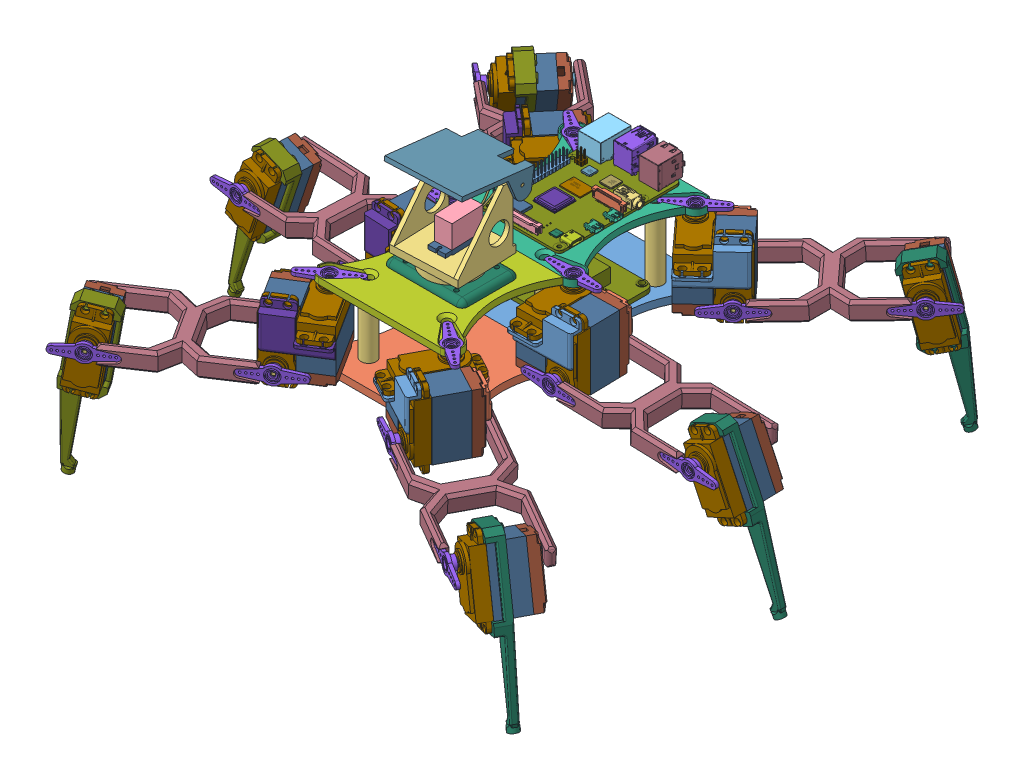
SolidWorks assembly 初号机, configuration 默认. Lengths in mm. (continued)
Components (placement in the parent): (continued)
- 舵机驱动板示意图-2: 舵机驱动板示意图 [默认] at (1.8543 8 4.9136) size (65 13 55)
Mates (geometry in assembly coordinates):
- 同心2: concentric anti-aligned: circle of bottom.step-1/Основание нижнее-0.step-1; circle of Втулка опорная-1
- 重合2: coincident anti-aligned: plane of bottom^666-1/Основание нижнее-0^bottom_666-1 through (0 5 85) normal (0 1 0); plane of Втулка опорная-1 through (-26.5949 5 115.9923) normal (0 -1 0)
- 同心3: concentric aligned: circle of bottom.step-1/Основание нижнее.step-1; circle of Втулка опорная-2
- 重合3: coincident anti-aligned: plane of bottom^666-1/Основание нижнее-0^bottom_666-1 through (0 5 85) normal (0 1 0); plane of Втулка опорная-2 through (-22.868 5 42.5) normal (0 -1 0)
- 重合4: coincident anti-aligned: plane of bottom^666-1/Основание нижнее^bottom_666-1 through (0 5 0) normal (0 1 0); plane of Втулка опорная-3 through (-26.5949 5 -30.9923) normal (0 -1 0)
- 同心5: concentric anti-aligned: cylinder of bottom.step-1/Основание нижнее.step-1; cylinder of Втулка опорная-3 through (-26.5949 50 -30.9923) axis (0 -1 0) radius 5.2
- 同心6: concentric aligned: circle of bottom.step-1/Основание нижнее.step-1; circle of Втулка опорная-4
- 重合5: coincident anti-aligned: plane of bottom^666-1/Основание нижнее^bottom_666-1 through (0 5 0) normal (0 1 0); plane of Втулка опорная-4 through (27.1009 5 -30.1473) normal (0 -1 0)
- 同心8: concentric anti-aligned: cylinder of bottom^666-1/Основание нижнее-0^bottom_666-1 through (27.1009 5 115.1473) axis (0 -1 0) radius 3; circle of Втулка опорная-6
- 重合6: coincident anti-aligned: plane of bottom^666-1/Основание нижнее-0^bottom_666-1 through (0 5 85) normal (0 1 0); plane of Втулка опорная-6 through (27.1009 5 115.1473) normal (0 -1 0)
- 重合7: coincident anti-aligned: plane of bottom^666-1/Основание нижнее^bottom_666-1 through (0 5 0) normal (0 1 0); plane of Втулка опорная-5 through (22.868 5 42.5) normal (0 -1 0)
- 同心9: concentric aligned: circle of Втулка опорная-5; circle of bottom.step-1/Основание нижнее.step-1
- 在位2: in place: plane of ? through (0 5 0) normal (0 1 0); plane of 零件4^初号机-1 through (0 5 0) normal (0 1 0); moOrthogonalPlaneRef_w of ? through (0 5 0) normal (0 1 0); plane of 零件4^初号机-1 through (0 5 0) normal (0 0 -1); plane of ? through (0 5 0) normal (0 1 0); plane of 零件4^初号机-1 through (0 5 0) normal (1 0 0); plane of ? through (0 5 0) normal (0 1 0); unknown of 零件4^初号机-1
- 重合21: coincident aligned: plane of ?; plane of ?
- 重合22: coincident aligned: moOrthogonalPlaneRef_w of bottom^666-1/Основание нижнее^bottom_666-1 through (0 5 0) normal (0 0 -1); plane of 零件4^666-1 through (0 5 0) normal (0 0 -1)
- 重合23: coincident anti-aligned: moOrthogonalPlaneRef_w of bottom^666-1/Основание нижнее^bottom_666-1 through (0 5 0) normal (-1 0 0); plane of 零件4^666-1 through (0 5 0) normal (1 0 0)
- 在位3: in place: plane of ? through (0 0 0) normal (0 -1 0); plane of 零件5^初号机-1 through (0 0 0) normal (0 -1 0); plane of ? through (0 0 0) normal (0 -1 0); plane of 零件5^初号机-1 through (0 0 0) normal (0 0 -1); plane of ? through (0 0 0) normal (0 -1 0); plane of 零件5^初号机-1 through (0 0 0) normal (-1 0 0); plane of ? through (0 0 0) normal (0 -1 0); unknown of 零件5^初号机-1
- 重合28: coincident aligned: plane of ?; plane of ?
- 重合29: coincident aligned: moOrthogonalPlaneRef_w of bottom^666-1/Основание нижнее^bottom_666-1 through (0 0 0) normal (0 0 -1); plane of 零件5^666-1 through (0 0 0) normal (0 0 -1)
- 重合30: coincident anti-aligned: moOrthogonalPlaneRef_w of bottom^666-1/Основание нижнее^bottom_666-1 through (0 0 0) normal (1 0 0); plane of 零件5^666-1 through (0 0 0) normal (-1 0 0)
- 同心10: concentric anti-aligned: cylinder of Втулка площадки-1 through (-42.5 5.3 -42.5) axis (0 -1 0) radius 2.5; circle of Подшипник-1
- 重合31: coincident anti-aligned: plane of Втулка площадки-1 through (-42.5 5.3 -42.5) normal (0 -1 0); circle of Подшипник-1
- 同心11: concentric aligned: circle of bottom^666-1/Основание нижнее^bottom_666-1; circle of Втулка площадки-1
- 重合33: coincident anti-aligned: plane of bottom^666-1/Основание нижнее^bottom_666-1 through (-42.5 3 -42.5) normal (0 1 0); plane of Подшипник-1 through (-42.5 3 -42.5) normal (0 -1 0)
- 同心12: concentric aligned: circle of Втулка площадки-2; circle of Подшипник-2
- 重合35: coincident anti-aligned: plane of Втулка площадки-2 through (42.5 5.5 -42.5) normal (0 -1 0); plane of Подшипник-2 through (42.5 5.5 -42.5) normal (0 1 0)
- 同心13: concentric aligned: circle of bottom^666-1/Основание нижнее^bottom_666-1; circle of Втулка площадки-2
- 重合36: coincident anti-aligned: plane of bottom^666-1/Основание нижнее^bottom_666-1 through (42.5 3 -42.5) normal (0 1 0); plane of Подшипник-2 through (42.5 3 -42.5) normal (0 -1 0)
- 同心14: concentric aligned: circle of Втулка площадки-3; circle of Подшипник-3
- 重合37: coincident anti-aligned: plane of Втулка площадки-3 through (42.5 7.5 42.5) normal (0 -1 0); plane of Подшипник-3 through (42.5 7.5 42.5) normal (0 1 0)
- 同心15: concentric aligned: circle of bottom^666-1/Основание нижнее^bottom_666-1; circle of Подшипник-3
- 重合38: coincident anti-aligned: plane of bottom^666-1/Основание нижнее-0^bottom_666-1 through (0 5 85) normal (0 1 0); plane of Подшипник-3 through (42.5 5 42.5) normal (0 -1 0)
- 同心17: concentric aligned: circle of bottom^666-1/Основание нижнее-0^bottom_666-1; circle of 底板转柱-4
- 同心18: concentric aligned: circle of bottom^666-1/Основание нижнее-0^bottom_666-1; circle of Подшипник-4
- 重合40: coincident anti-aligned: plane of 底板转柱-4 through (42.5 5.5 127.5) normal (0 -1 0); plane of Подшипник-4 through (42.5 5.5 127.5) normal (0 1 0)
- 重合41: coincident anti-aligned: plane of bottom^666-1/Основание нижнее-0^bottom_666-1 through (42.5 3 127.5) normal (0 1 0); plane of Подшипник-4 through (42.5 3 127.5) normal (0 -1 0)
- 同心19: concentric aligned: circle of 底板转柱-5; circle of Подшипник-6
- 重合43: coincident anti-aligned: plane of 底板转柱-5 through (-42.5 5.3 127.5) normal (0 -1 0); plane of Подшипник-6 through (-42.5 5.3 127.5) normal (0 1 0)
- 同心20: concentric aligned: circle of bottom^666-1/Основание нижнее-0^bottom_666-1; circle of 底板转柱-5
- 重合44: coincident anti-aligned: plane of bottom^666-1/Основание нижнее-0^bottom_666-1 through (-42.5 3 127.5) normal (0 1 0); plane of Подшипник-6 through (-42.5 3 127.5) normal (0 -1 0)
- 同心21: concentric aligned: circle of Подшипник-5; circle of 底板转柱-6
- 重合45: coincident anti-aligned: plane of Подшипник-5 through (-42.5 5.5 42.5) normal (0 1 0); plane of 底板转柱-6 through (-42.5 5.5 42.5) normal (0 -1 0)
- 同心22: concentric aligned: circle of Подшипник-5; circle of bottom^666-1/Основание нижнее^bottom_666-1
- 重合46: coincident anti-aligned: plane of bottom^666-1/Основание нижнее^bottom_666-1 through (-42.5 3 42.5) normal (0 1 0); plane of Подшипник-5 through (-42.5 3 42.5) normal (0 -1 0)
- 同心36: concentric anti-aligned: circle of Рычаг-7; circle of Servo MG955-1/Втулка-1
- 重合72: coincident anti-aligned: plane of Рычаг-7 through (-42.5 51.5 127.5) normal (0 -1 0); plane of Servo MG955-1/MG995齿轮-1 through (-42.5 51.5 127.5) normal (0 1 0)
- 重合83: coincident anti-aligned: plane of Servo MG955-1/MG995中板-1 through (-56.5553 34.5 124.2521) normal (-0.84292 0 0.538039); plane of 腿1-2/Servo MG955-2/MG995中板-1 through (-40.6024 4.85 149.2447) normal (0.84292 0 -0.538039)
- 重合84: coincident aligned: plane of Servo MG955-1/MG995中板-1 through (-34.6302 34.5 158.6011) normal (0.538039 0 0.84292); plane of 腿1-2/Servo MG955-2/MG995前板-1 through (-43.1437 35.4 164.0353) normal (0.538039 0 0.84292)
- 重合85: coincident aligned: plane of Servo MG955-1/MG995前板-1 through (-31.6047 45.6 144.5691) normal (0 1 0); plane of 腿1-2/Servo MG955-2/MG995中板-1 through (-40.6024 45.6 149.2447) normal (0 1 0)
- 重合86: coincident anti-aligned: plane of 底板支柱-4 through (27.1009 50 -30.1473) normal (0 1 0); plane of top(3)-1/top(3)^top(3)-2/^top(3)_top(3)-1/Основание нижнее^_top(3)_top(3)-1 through (0 50 0) normal (0 -1 0)
- 同心37: concentric anti-aligned: circle of 底板支柱-4; circle of top(3)-1/top(3)^top(3)-2/^top(3)_top(3)-1/Основание нижнее^_top(3)_top(3)-1
- 同心38: concentric anti-aligned: circle of 底板支柱-1; circle of top(3)-1/top(3)^top(3)-2/_private_var_mobile_Containers_Data_Application_327FD876-EF9E-4CCE-9D75-9D16AF0753A7_tmp_B33AE067-E3AF-4F21-8502-7502B160869B.tmp(2)^top(3)_top(3)-1
- 同心39: concentric aligned: circle of top(3)-1/top(3)^top(3)-2/_private_var_mobile_Containers_Data_Application_327FD876-EF9E-4CCE-9D75-9D16AF0753A7_tmp_B33AE067-E3AF-4F21-8502-7502B160869B.tmp(2)^top(3)_top(3)-1; circle of 舵机配件-7
- 重合87: coincident anti-aligned: plane of top(3)-1/top(3)^top(3)-2/_private_var_mobile_Containers_Data_Application_327FD876-EF9E-4CCE-9D75-9D16AF0753A7_tmp_B33AE067-E3AF-4F21-8502-7502B160869B.tmp(2)^top(3)_top(3)-1 through (0 51.5 0) normal (0 1 0); plane of 舵机配件-7 through (-42.5 51.5 127.5) normal (0 -1 0)
- 平行1: parallel aligned: line of top(3)-1/top(3)^top(3)-2/_private_var_mobile_Containers_Data_Application_327FD876-EF9E-4CCE-9D75-9D16AF0753A7_tmp_B33AE067-E3AF-4F21-8502-7502B160869B.tmp(2)^top(3)_top(3)-1 through (-42.5 51.5 127.5) axis (0.81018 0 -0.586182); line of 舵机配件-7 through (-55.8921 53.8 137.1895) axis (0.81018 0 -0.586182)
- 同心40: concentric aligned: circle of top(3)-1/top(3)^top(3)-2/_private_var_mobile_Containers_Data_Application_327FD876-EF9E-4CCE-9D75-9D16AF0753A7_tmp_B33AE067-E3AF-4F21-8502-7502B160869B.tmp(2)^top(3)_top(3)-1; circle of 舵机配件-6
- 重合89: coincident anti-aligned: plane of top(3)-1/top(3)^top(3)-2/_private_var_mobile_Containers_Data_Application_327FD876-EF9E-4CCE-9D75-9D16AF0753A7_tmp_B33AE067-E3AF-4F21-8502-7502B160869B.tmp(2)^top(3)_top(3)-1 through (0 51.5 0) normal (0 1 0); plane of 舵机配件-6 through (42.5 51.5 127.5) normal (0 -1 0)
- 平行2: parallel aligned: line of top(3)-1/top(3)^top(3)-2/_private_var_mobile_Containers_Data_Application_327FD876-EF9E-4CCE-9D75-9D16AF0753A7_tmp_B33AE067-E3AF-4F21-8502-7502B160869B.tmp(2)^top(3)_top(3)-1 through (34.4656 51.5 121.055) axis (0.780043 0 0.625726); line of 舵机配件-6 through (29.6061 53.8 117.1569) axis (0.780043 0 0.625726)
- 同心41: concentric aligned: circle of top(3)-1/top(3)^top(3)-2/^top(3)_top(3)-1/Основание нижнее^_top(3)_top(3)-1; circle of 舵机配件-8
- 重合91: coincident anti-aligned: plane of top(3)-1/top(3)^top(3)-2/^top(3)_top(3)-1/Основание нижнее^_top(3)_top(3)-1 through (0 51.5 0) normal (0 1 0); plane of 舵机配件-8 through (42.5 51.5 42.5) normal (0 -1 0)
- 平行3: parallel aligned: line of top(3)-1/top(3)^top(3)-2/^top(3)_top(3)-1/Основание нижнее^_top(3)_top(3)-1 through (42.5 51.5 42.5) axis (-1 0 0); line of 舵机配件-8 through (59.0298 53.8 42.5) axis (-1 0 0)
- 同心42: concentric anti-aligned: circle of top(3)-1/top(3)^top(3)-2/^top(3)_top(3)-1/Основание нижнее^_top(3)_top(3)-1; circle of 舵机配件-5
- 重合95: coincident anti-aligned: plane of top(3)-1/top(3)^top(3)-2/^top(3)_top(3)-1/Основание нижнее^_top(3)_top(3)-1 through (0 51.5 0) normal (0 1 0); plane of 舵机配件-5 through (-42.5 51.5 42.5) normal (0 -1 0)
- 平行4: parallel aligned: line of top(3)-1/top(3)^top(3)-2/^top(3)_top(3)-1/Основание нижнее^_top(3)_top(3)-1 through (-42.5 51.5 42.5) axis (1 0 0); line of 舵机配件-5 through (-59.0298 53.8 42.5) axis (1 0 0)
- 同心44: concentric aligned: circle of top(3)-1/top(3)^top(3)-2/^top(3)_top(3)-1/Основание нижнее^_top(3)_top(3)-1; circle of 舵机配件-4
- 重合97: coincident anti-aligned: plane of top(3)-1/top(3)^top(3)-2/^top(3)_top(3)-1/Основание нижнее^_top(3)_top(3)-1 through (0 51.5 0) normal (0 1 0); plane of 舵机配件-4 through (-42.5 51.5 -42.5) normal (0 -1 0)
- 平行5: parallel aligned: line of top(3)-1/top(3)^top(3)-2/^top(3)_top(3)-1/Основание нижнее^_top(3)_top(3)-1 through (-42.5 51.5 -42.5) axis (0.81018 0 0.586182); line of 舵机配件-4 through (-55.8921 53.8 -52.1895) axis (0.81018 0 0.586182)
- 同心45: concentric aligned: circle of top(3)-1/top(3)^top(3)-2/^top(3)_top(3)-1/Основание нижнее^_top(3)_top(3)-1; circle of 舵机配件-3
- 重合99: coincident anti-aligned: plane of top(3)-1/top(3)^top(3)-2/^top(3)_top(3)-1/Основание нижнее^_top(3)_top(3)-1 through (0 51.5 0) normal (0 1 0); plane of 舵机配件-3 through (42.5 51.5 -42.5) normal (0 -1 0)
- 平行6: parallel anti-aligned: line of top(3)-1/top(3)^top(3)-2/^top(3)_top(3)-1/Основание нижнее^_top(3)_top(3)-1 through (42.5 51.5 -42.5) axis (-0.783045 0 0.621965); line of 舵机配件-3 through (29.5564 53.8 -32.2191) axis (0.783045 0 -0.621965)
- 重合100: coincident anti-aligned: plane of 腿1-2/Servo MG955-2/MG995前板-1 through (-43.1437 35.4 164.0353) normal (0.538039 0 0.84292); plane of 固定件1-1 through (-26.1167 13.85 153.1669) normal (-0.538039 0 -0.84292)
- 同心46: concentric aligned: circle of 腿1-2/Servo MG955-2/MG995前板-1; circle of 固定件1-1
- 重合102: coincident anti-aligned: line of Servo MG955-1/MG995中板-1 through (-34.6302 34.5 158.6011) axis (0.84292 0 -0.538039); line of 固定件1-1 through (-17.6032 34.5 147.7327) axis (-0.84292 0 0.538039)
- 重合103: coincident anti-aligned: plane of 腿1-2/Servo MG955-2/MG995后板-1 through (-64.2348 25.235 130.9928) normal (-0.538039 0 -0.84292); plane of 固定件2-1 through (-47.2078 13.85 120.1244) normal (0.538039 0 0.84292)
- 同心47: concentric aligned: circle of 腿1-2/Servo MG955-2/MG995后板-1; circle of 固定件2-1
- 同心48: concentric anti-aligned: circle of 腿1-2/Servo MG955-2/MG995后板-1; circle of 固定件2-1
- 重合106: coincident anti-aligned: plane of 舵机配件-5 through (-42.5 51.5 42.5) normal (0 -1 0); plane of Servo MG955-2/MG995齿轮-1 through (-42.5 51.5 42.5) normal (0 1 0)
- 同心49: concentric anti-aligned: circle of 舵机配件-5; circle of Servo MG955-2/MG995齿轮-1
- 重合107: coincident anti-aligned: plane of 腿1-3/Servo MG955-2/MG995中板-1 through (-53.5221 4.85 61.34) normal (0.998835 0 0.048264); plane of Servo MG955-2/MG995中板-1 through (-52.0911 34.5 31.7245) normal (-0.998835 0 -0.048264)
- 重合108: coincident aligned: plane of 腿1-3/Servo MG955-2/MG995前板-1 through (-64.1461 35.4 71.9396) normal (-0.048264 0 0.998835); plane of Servo MG955-2/MG995中板-1 through (-54.0579 34.5 72.4271) normal (-0.048264 0 0.998835)
- 重合109: coincident aligned: plane of 腿1-3/Servo MG955-2/MG995中板-1 through (-53.5221 45.6 61.34) normal (0 1 0); plane of Servo MG955-2/MG995前板-1 through (-43.4773 45.6 62.7264) normal (0 1 0)
- 重合110: coincident anti-aligned: plane of 腿1-3/Servo MG955-2/MG995前板-1 through (-64.1461 35.4 71.9396) normal (-0.048264 0 0.998835); plane of 固定件1-2 through (-43.9696 13.85 72.9145) normal (0.048264 0 -0.998835)
- 同心50: concentric aligned: circle of 腿1-3/Servo MG955-2/MG995前板-1; circle of 固定件1-2
- 重合113: coincident anti-aligned: line of Servo MG955-2/MG995中板-1 through (-54.0579 34.5 72.4271) axis (0.998835 0 0.048264); line of 固定件1-2 through (-33.8814 34.5 73.402) axis (-0.998835 0 -0.048264)
- 同心51: concentric aligned: circle of 腿1-3/Servo MG955-2/MG995后板-1; circle of 固定件2-2
- 同心52: concentric anti-aligned: circle of 腿1-2/Servo MG955-2/MG995后板-1; circle of 固定件2-1
- 重合119: coincident anti-aligned: plane of 腿1-3/Servo MG955-2/MG995后板-1 through (-72.4075 45.6 33.6462) normal (0.048264 0 -0.998835); plane of 固定件2-2 through (-42.1428 13.85 35.1086) normal (-0.048264 0 0.998835)
- 同心54: concentric anti-aligned: circle of 腿1-3/Servo MG955-2/MG995后板-1; circle of 固定件2-2
- 重合126: coincident anti-aligned: plane of 腿1-4/Servo MG955-2/MG995前板-1 through (-77.5718 35.4 -32.2426) normal (-0.644628 0 0.764496); plane of 固定件1-3 through (-62.1289 13.85 -19.2211) normal (0.644628 0 -0.764496)
- 同心57: concentric aligned: circle of 腿1-4/Servo MG955-2/MG995前板-1; circle of 固定件1-3
- 同心58: concentric aligned: circle of 腿1-4/Servo MG955-2/MG995前板-1; circle of 固定件1-3
- 重合130: coincident anti-aligned: plane of 腿1-4/Servo MG955-2/MG995后板-1 through (-52.3023 25.235 -62.2108) normal (0.644628 0 -0.764496); plane of 固定件2-3 through (-36.8595 13.85 -49.1893) normal (-0.644628 0 0.764496)
- 同心59: concentric anti-aligned: circle of 腿1-4/Servo MG955-2/MG995后板-1; circle of 固定件2-3
- 同心60: concentric aligned: circle of 腿1-4/Servo MG955-2/MG995后板-1; circle of 固定件2-3
- 同心61: concentric anti-aligned: circle of 舵机配件-6; circle of Servo MG955-4/MG995齿轮-1
- 重合135: coincident anti-aligned: plane of 舵机配件-6 through (42.5 51.5 127.5) normal (0 -1 0); plane of Servo MG955-4/MG995齿轮-1 through (42.5 51.5 127.5) normal (0 1 0)
- 重合136: coincident anti-aligned: plane of Servo MG955-4/MG995中板-1 through (56.2471 34.5 123.1278) normal (0.883614 0 0.468216); plane of 腿2-2/Servo MG955-2/MG995中板-1 through (42.3645 4.85 149.3269) normal (-0.883614 0 -0.468216)
- 重合137: coincident aligned: plane of Servo MG955-4/MG995前板-1 through (33.0186 45.6 145.3932) normal (0 1 0); plane of 腿2-2/Servo MG955-2/MG995中板-1 through (60.2135 45.6 158.7849) normal (0 1 0)
- 重合138: coincident aligned: plane of Servo MG955-4/MG995中板-1 through (19.3183 34.5 149.6771) normal (-0.468216 0 0.883614); plane of 腿2-2/Servo MG955-2/MG995前板-1 through (46.0918 35.4 163.864) normal (-0.468216 0 0.883614)
- 重合139: coincident anti-aligned: plane of 腿2-2/Servo MG955-2/MG995前板-1 through (46.0918 35.4 163.864) normal (-0.468216 0 0.883614); plane of 镜向固定件1-1 through (28.2428 13.85 154.406) normal (0.468216 0 -0.883614)
- 同心62: concentric anti-aligned: circle of 腿2-2/Servo MG955-2/MG995前板-1; circle of 镜向固定件1-1
- 同心63: concentric anti-aligned: circle of 腿2-2/Servo MG955-2/MG995前板-1; circle of 镜向固定件1-1
- 重合143: coincident anti-aligned: plane of 腿2-2/Servo MG955-2/MG995后板-1 through (64.4459 25.235 129.2263) normal (0.468216 0 -0.883614); plane of 镜向固定件2-1 through (46.5969 13.85 119.7684) normal (-0.468216 0 0.883614)
- 同心64: concentric anti-aligned: circle of 腿2-2/Servo MG955-2/MG995后板-1; circle of 镜向固定件2-1
- 同心65: concentric aligned: circle of 腿2-2/Servo MG955-2/MG995后板-1; circle of 镜向固定件2-1
- 同心66: concentric anti-aligned: circle of 舵机配件-8; circle of Servo MG955-5/MG995齿轮-1
- 重合146: coincident anti-aligned: plane of 舵机配件-8 through (42.5 51.5 42.5) normal (0 -1 0); circle of Servo MG955-5/MG995齿轮-1
- 重合147: coincident anti-aligned: plane of 腿2-1/Servo MG955-2/MG995中板-1 through (53.0061 4.85 61.6325) normal (-0.999777 0 0.021104); plane of Servo MG955-5/MG995中板-1 through (52.3804 34.5 31.9891) normal (0.999777 0 -0.021104)
- 重合148: coincident aligned: plane of 腿2-1/Servo MG955-2/MG995前板-1 through (63.3381 35.4 72.5169) normal (0.021104 0 0.999777); plane of Servo MG955-5/MG995中板-1 through (33.0449 34.5 73.1564) normal (0.021104 0 0.999777)
- 重合149: coincident aligned: plane of 腿2-1/Servo MG955-2/MG995中板-1 through (73.2016 45.6 61.2062) normal (0 1 0); plane of Servo MG955-5/MG995前板-1 through (42.9274 45.6 62.7455) normal (0 1 0)
- 重合151: coincident anti-aligned: plane of 腿2-1/Servo MG955-2/MG995前板-1 through (63.3381 35.4 72.5169) normal (0.021104 0 0.999777); plane of 镜向固定件1-2 through (43.1426 13.85 72.9432) normal (-0.021104 0 -0.999777)
- 同心67: concentric anti-aligned: circle of 腿2-1/Servo MG955-2/MG995前板-1; circle of 镜向固定件1-2
- 同心68: concentric anti-aligned: circle of 腿2-1/Servo MG955-2/MG995前板-1; circle of 镜向固定件1-2
- 重合154: coincident anti-aligned: plane of 腿2-1/Servo MG955-2/MG995后板-1 through (62.5108 25.235 33.3256) normal (-0.021104 0 -0.999777); plane of 镜向固定件2-2 through (42.3153 13.85 33.7519) normal (0.021104 0 0.999777)
- 同心69: concentric aligned: circle of 腿2-1/Servo MG955-2/MG995后板-1; circle of 镜向固定件2-2
- 同心70: concentric anti-aligned: circle of 腿2-1/Servo MG955-2/MG995后板-1; circle of 镜向固定件2-2
- 重合157: coincident anti-aligned: plane of 舵机配件-3 through (42.5 51.5 -42.5) normal (0 -1 0); plane of Servo MG955-6/MG995齿轮-1 through (42.5 51.5 -42.5) normal (0 1 0)
- 同心71: concentric anti-aligned: circle of 舵机配件-3; circle of Servo MG955-6/MG995齿轮-1
- 重合158: coincident anti-aligned: plane of Servo MG955-6/MG995中板-1 through (43.0145 34.5 -56.9165) normal (0.73852 0 -0.674231); plane of 腿2-3/Servo MG955-2/MG995中板-1 through (63.0054 4.85 -35.0194) normal (-0.73852 0 0.674231)
- 重合159: coincident aligned: plane of Servo MG955-6/MG995中板-1 through (55.5713 34.5 -13.2023) normal (0.674231 0 0.73852); plane of 腿2-3/Servo MG955-2/MG995前板-1 through (77.9484 35.4 -33.6315) normal (0.674231 0 0.73852)
- 重合160: coincident aligned: plane of Servo MG955-6/MG995前板-1 through (56.1532 45.6 -27.545) normal (0 1 0); plane of 腿2-3/Servo MG955-2/MG995中板-1 through (77.9235 45.6 -48.6388) normal (0 1 0)
- 重合161: coincident anti-aligned: plane of 腿2-3/Servo MG955-2/MG995前板-1 through (77.9484 35.4 -33.6315) normal (0.674231 0 0.73852); plane of 镜向固定件1-3 through (63.0303 13.85 -20.0121) normal (-0.674231 0 -0.73852)
- 同心72: concentric anti-aligned: circle of 腿2-3/Servo MG955-2/MG995前板-1; circle of 镜向固定件1-3
- 同心73: concentric anti-aligned: circle of 腿2-3/Servo MG955-2/MG995前板-1; circle of 镜向固定件1-3
- 重合165: coincident aligned: plane of Servo MG955-4/MG995前板-1 through (33.0186 45.6 145.3932) normal (0 1 0); plane of 腿2-2/Servo MG955-2/MG995中板-1 through (60.2135 45.6 158.7849) normal (0 1 0)
- 平行9: parallel anti-aligned: plane of Servo MG955-4/MG995中板-1 through (56.2471 34.5 123.1278) normal (0.883614 0 0.468216); plane of 腿2-2/Servo MG955-2/MG995中板-1 through (42.3645 4.85 149.3269) normal (-0.883614 0 -0.468216)
- 重合169: coincident anti-aligned: plane of Servo MG955-4/MG995中板-1 through (56.2471 34.5 123.1278) normal (0.883614 0 0.468216); plane of 腿2-2/Servo MG955-2/MG995中板-1 through (42.3645 4.85 149.3269) normal (-0.883614 0 -0.468216)
- 重合170: coincident anti-aligned: plane of 腿2-3/Servo MG955-2/MG995后板-1 through (51.5186 25.235 -62.5815) normal (-0.674231 0 -0.73852); plane of 镜向固定件2-3 through (36.6005 13.85 -48.9621) normal (0.674231 0 0.73852)
- 同心74: concentric aligned: circle of 腿2-3/Servo MG955-2/MG995后板-1; circle of 镜向固定件2-3
- 同心75: concentric anti-aligned: circle of 腿2-3/Servo MG955-2/MG995后板-1; circle of 镜向固定件2-3
- 重合173: coincident anti-aligned: plane of 舵机配件-4 through (-42.5 51.5 -42.5) normal (0 -1 0); plane of Servo MG955-7/MG995齿轮-1 through (-42.5 51.5 -42.5) normal (0 1 0)
- 同心76: concentric aligned: circle of 舵机配件-4; circle of Servo MG955-7/MG995齿轮-1
- 重合174: coincident anti-aligned: plane of 腿1-4/Servo MG955-2/MG995中板-1 through (-62.695 4.85 -34.2177) normal (0.764496 0 0.644628); plane of Servo MG955-7/MG995中板-1 through (-43.5817 34.5 -56.8851) normal (-0.764496 0 -0.644628)
- 重合175: coincident aligned: plane of 腿1-4/Servo MG955-2/MG995中板-1 through (-62.695 45.6 -34.2177) normal (0 1 0); plane of Servo MG955-7/MG995前板-1 through (-55.5537 45.6 -27.0189) normal (0 1 0)
- 重合177: coincident anti-aligned: plane of 固定件1-3 through (-62.1289 13.85 -19.2211) normal (0.644628 0 -0.764496); plane of Servo MG955-7/MG995中板-1 through (-69.8503 34.5 -25.7318) normal (-0.644628 0 0.764496)
- 重合178: coincident anti-aligned: plane of top(3)-1/top(3)^top(3)-2/_private_var_mobile_Containers_Data_Application_327FD876-EF9E-4CCE-9D75-9D16AF0753A7_tmp_B33AE067-E3AF-4F21-8502-7502B160869B.tmp(2)^top(3)_top(3)-1 through (0 55 85) normal (0 1 0); plane of 云台2号机 -1/云台1-1 through (0 55 85) normal (0 -1 0)
- 重合182: coincident anti-aligned: line of top(3)-1/top(3)^top(3)-2/_private_var_mobile_Containers_Data_Application_327FD876-EF9E-4CCE-9D75-9D16AF0753A7_tmp_B33AE067-E3AF-4F21-8502-7502B160869B.tmp(2)^top(3)_top(3)-1 through (-42.8869 55 85) axis (1 0 0); line of 云台2号机 -1/云台1-1 through (17.5 55 85) axis (-1 0 0)
- 重合183: coincident aligned: line of top(3)-1/top(3)^top(3)-2/_private_var_mobile_Containers_Data_Application_327FD876-EF9E-4CCE-9D75-9D16AF0753A7_tmp_B33AE067-E3AF-4F21-8502-7502B160869B.tmp(2)^top(3)_top(3)-1 through (0 55 49.99) axis (0 0 1); line of 云台2号机 -1/云台1-1 through (0 55 71) axis (0 0 1)
- 重合187: coincident anti-aligned: plane of top(3)-1/top(3)^top(3)-2/^top(3)_top(3)-1/Основание нижнее^_top(3)_top(3)-1 through (0 55 0) normal (0 1 0); plane of rpi4b-1/rpi4b(2)^rpi4b-1/PCB, RPi4ModelB^rpi4b(2)_rpi4b-1 through (0 55 -4.664) normal (0 -1 0)
- 重合188: coincident aligned: line of top(3)-1/top(3)^top(3)-2/^top(3)_top(3)-1/Основание нижнее^_top(3)_top(3)-1 through (32.7407 55 5.336) axis (-1 0 0); line of rpi4b-1/rpi4b(2)^rpi4b-1/PCB, RPi4ModelB^rpi4b(2)_rpi4b-1 through (24.5 55 5.336) axis (-1 0 0)
- 重合189: coincident anti-aligned: line of top(3)-1/top(3)^top(3)-2/^top(3)_top(3)-1/Основание нижнее^_top(3)_top(3)-1 through (0 55 -50) axis (0 0 1); line of rpi4b-1/rpi4b(2)^rpi4b-1/PCB, RPi4ModelB^rpi4b(2)_rpi4b-1 through (0 55 34.336) axis (0 0 -1)
- 同心80: concentric aligned: circle of top(3)-1/top(3)^top(3)-2/^top(3)_top(3)-1/Основание нижнее^_top(3)_top(3)-1; circle of rpi4b-1/rpi4b(2)^rpi4b-1/PCB, RPi4ModelB^rpi4b(2)_rpi4b-1
- 同心81: concentric aligned: circle of top(3)-1/top(3)^top(3)-2/^top(3)_top(3)-1/Основание нижнее^_top(3)_top(3)-1; circle of rpi4b-1/rpi4b(2)^rpi4b-1/PCB, RPi4ModelB^rpi4b(2)_rpi4b-1
- 重合191: coincident anti-aligned: plane of bottom^666-1/Основание нижнее^bottom_666-1 through (0 5 0) normal (0 1 0); plane of 舵机驱动板示意图-2 through (1.8543 5 4.9136) normal (0 -1 0)
- 平行10: parallel aligned: line of bottom^666-1/Основание нижнее^bottom_666-1 through (-42.5 5 -50) axis (1 0 0); line of 舵机驱动板示意图-2 through (-27 8 -23.6747) axis (1 0 0)
- 重合196: coincident aligned: line of bottom^666-1/Основание нижнее^bottom_666-1 through (-35.6301 5 3.8253) axis (1 0 0); line of 舵机驱动板示意图-2 through (-32.5 5 3.8253) axis (1 0 0)
- 重合197: coincident anti-aligned: line of bottom^666-1/Основание нижнее^bottom_666-1 through (0 5 50) axis (0 0 -1); line of 舵机驱动板示意图-2 through (0 5 -23.6747) axis (0 0 1)
- 同心89: concentric aligned: circle of bottom^666-1/Основание нижнее^bottom_666-1; circle of 舵机驱动板示意图-2
- 同心90: concentric aligned: circle of bottom^666-1/Основание нижнее^bottom_666-1; circle of 舵机驱动板示意图-2
